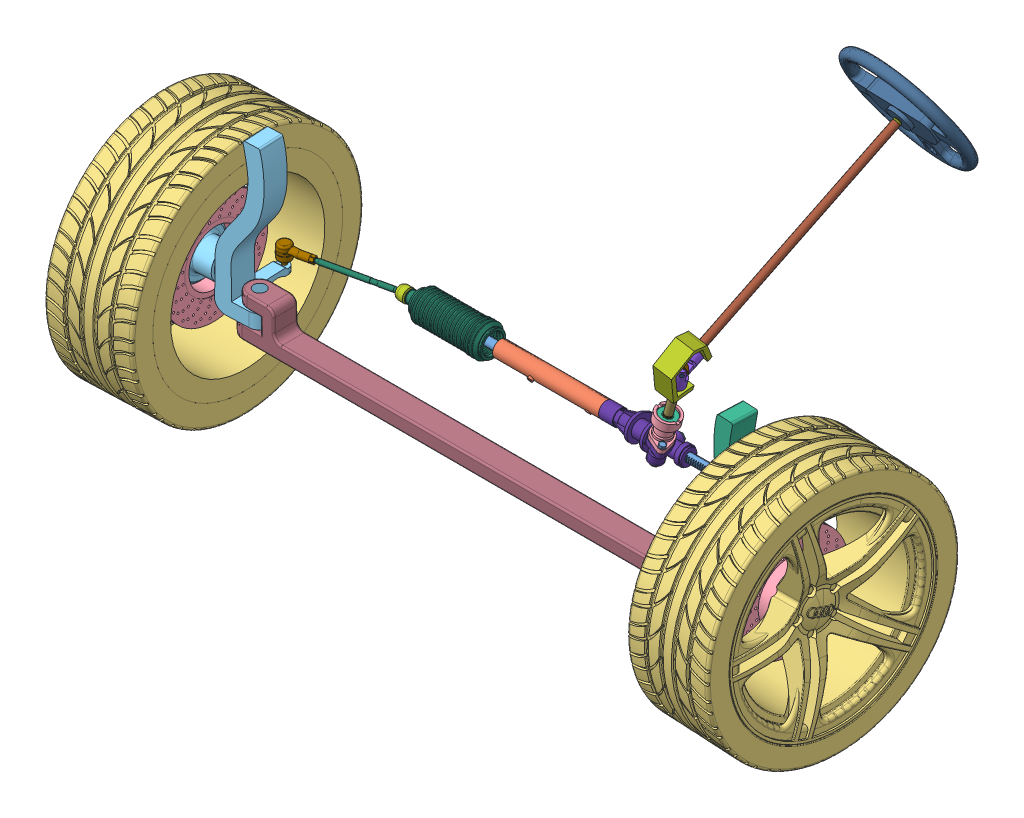
SolidWorks assembly HỆ THỐNG LÁI, configuration Default. Lengths in mm.
Overall size (1991.38 1196.91 1377.29).
45 component instances, 34 part files, 99 mates.
Components (placement in the parent):
- formed hex screw_am-1: formed hex screw_am [B18.2.3.2M - Formed hex screw, M10 x 1.5 x 25 --25WS] at (203.2147 96.225 194.8951) x (-0.267944 -0.963434 0) z (0.029399 -0.008176 0.999534) size (31.63 18.48 16)
- formed hex screw_am-2: formed hex screw_am [B18.2.3.2M - Formed hex screw, M10 x 1.5 x 25 --25WS] at (249.0045 83.4902 243.5967) x (-0.267944 -0.963434 0) z (0.097823 -0.027206 0.994832) size (31.63 18.48 16)
- THƯỚC LÁI-3: THƯỚC LÁI [Default] at (-246.9846 43.7433 199.2709) x (1 0 0) z (0 -0.882001 -0.471248) size (295 48.35 43.5)
- BÁNH XE-1: BÁNH XE [Varsayılan] at (-55.7357 64.8163 360.7964) x (0.047772 -0.300245 -0.952665) z (-0.016934 -0.95386 0.299772) size (668.92 273.92 668.92)
- ĐĨA THẮNG-2: ĐĨA THẮNG [Default] at (-852.1937 65.1305 399.9751) x (0.004037 0.995257 0.097198) z (0.035256 -0.09728 0.994632) size (303 56.33 303)
- BÁNH XE-2: BÁNH XE [Varsayılan] at (-42.761 64.6537 371.2368) x (-0.023989 -0.748 -0.663265) z (-0.02615 0.663699 -0.747543) size (668.92 273.92 668.92)
- KHUNG TREO R-1: KHUNG TREO R [Default] at (-765.1865 65.0792 396.886) x (-0.99937 0.000589 0.035482) z (0.03547 -0.014236 0.999269) size (231.48 449.46 221.1)
- KHUNG TREO L-1: KHUNG TREO L [Default] at (670.2109 63.4994 397.6144) x (0.998715 -0.001812 0.050652) z (0.050673 0.014132 -0.998615) size (231.48 449.46 221.1)
- ĐĨA THẮNG-3: ĐĨA THẮNG [Default] at (753.1662 63.349 401.8216) x (-0.048602 -0.317762 0.946924) z (-0.01438 0.948169 0.317441) size (303 56.33 303)
- CACDANG 5-1: CACDANG 5 [Default] at (259.0901 291.6158 242.3294) x (-0.055622 -0.503507 0.862199) z (0.959177 -0.26676 -0.093904) size (119.51 136.21 49)
- CACDANG 1-2: CACDANG 1 [Default] at (278.0374 289.9791 179.6097) x (-0.173357 0.85529 0.488289) z (-0.055622 -0.503507 0.862199) size (40 40 56)
- CACDANG 2-2: CACDANG 2 [Default] at (284.0824 264.425 226.5167) x (0.640489 0.474538 -0.603811) z (-0.748145 0.208069 -0.630068) size (23 23 23)
- CACDANG 3-1: CACDANG 3 [Default] at (260.5158 270.9792 206.6695) x (0.65777 0.107664 -0.745484) z (0.748145 -0.208069 0.630068) size (10 10 40.8)
- CACDANG 4-1: CACDANG 4 [Default] at (278.9459 249.712 209.5051) x (0.851053 0.379608 -0.362775) z (-0.173357 0.85529 0.488289) size (10 10 14.2)
- CACDANG 4-2: CACDANG 4 [Default] at (274.4733 271.7785 222.103) x (0.851053 0.379608 -0.362775) z (-0.173357 0.85529 0.488289) size (10 10 14.2)
- TRỤC NỐI TRỤC VÍT-2: TRỤC NỐI TRỤC VÍT [Default] at (240.646 141.5713 219.2709) x (0.960852 -0.267226 0.073168) z (0.267944 0.963434 0) size (20 20 100)
- CACDANG 1-3: CACDANG 1 [Default] at (263.1533 222.4998 219.2709) x (0.748145 -0.208069 0.630068) z (0.267944 0.963434 0) size (40 40 56)
- KHUNG GẦM-3: KHUNG GẦM [Default] at (-47.6162 -67.6316 359.9452) x (0.999999 -0.001094 0.000037) z (-0.001093 -0.999898 -0.014206) size (1446 67 117)
- CHỐT HÃM-6: CHỐT HÃM [Default] at (625.5096 48.1445 395.1288) x (0.999999 -0.001094 0.000016) z (-0.001093 -0.999898 -0.014206) size (33.5 33.5 117)
- CHỐT HÃM-5: CHỐT HÃM [Default] at (-720.4896 49.6169 395.0791) x (0.999999 -0.001094 0.000016) z (-0.001093 -0.999898 -0.014206) size (33.5 33.5 117)
- ROTUYN TRONG-1: ROTUYN TRONG [Default] at (-504.6777 43.5088 197.2103) x (-0.9763 -0.000113 0.216421) z (0.160624 -0.670575 0.724244) size (257.66 24 24)
- ROTUYN TRONG-2: ROTUYN TRONG [Default] at (412.1674 43.7741 196.4187) x (0.97478 -0.002427 0.223157) z (0.130993 0.815786 -0.563324) size (257.66 24 24)
- TRỤC VÔ LĂNG 2-3: TRỤC VÔ LĂNG 2 [Default] at (283.9585 343.601 87.7844) x (0.989756 0.085913 0.114023) z (0.055622 0.503507 -0.862199) size (20 20 532)
- VỎ CƠ CẤU LÁI-2: VỎ CƠ CẤU LÁI [Default] at (41.4337 43.7433 199.2709) size (236.3 72.67 100.51)
- TRỤC VÍT-1: TRỤC VÍT [Default] at (206.441 18.5819 219.2709) x (0.686426 -0.190854 -0.701708) z (0.67605 -0.188019 0.712465) size (25.52 146.66 25.52)
- THANH RĂNG-2: THANH RĂNG [Default] at (402.7364 43.7433 199.2709) x (0 -1 -0.000036) z (-1 0 0) size (38 38 898)
- Ổ BI NHỎ-1: Ổ BI NHỎ [Default] at (206.4223 18.5148 219.2709) x (-0.956047 0.26589 0.123602) z (-0.119083 0.033119 -0.992332) size (26 8 26)
- NẮP Ổ BI-1: NẮP Ổ BI [Default] at (201.9775 2.5329 219.2709) x (0.963402 -0.267884 0.009757) z (-0.0094 0.002614 0.999952) size (30.59 16.59 30.59)
- VỎ TRỤC VÍT-1: VỎ TRỤC VÍT [Default] at (224.4762 83.4302 219.2711) x (-0.013584 0.003742 0.999901) z (-0.963339 0.267918 -0.01409) size (68.03 72.52 68.21)
- Ổ BI HÃM-1: Ổ BI HÃM [Default] at (219.596 65.8829 219.2709) x (0.843571 -0.234609 -0.483059) z (0.465396 -0.129433 0.875588) size (37.58 11 37.58)
- Ổ BI LỚN-1: Ổ BI LỚN [Default] at (239.2278 136.4722 219.273) x (-0.596204 0.16584 -0.785517) z (-0.267944 -0.963435 -0.000034) size (47 47 14)
- KHỚP CẦU 3-1: KHỚP CẦU 3 [Default] at (408.7364 43.7474 198.8734) x (-1 0 0) z (0 -0.010312 0.999947) size (48.52 36 36)
- KHỚP CẦU 3-2: KHỚP CẦU 3 [Default] at (-501.2636 43.5076 199.5909) x (1 0 0) z (0 0.593004 -0.8052) size (48.52 36 36)
- KHỚP CẦU-1: KHỚP CẦU [Default] at (408.8899 43.7474 198.8734) x (0 -0.967498 -0.252877) z (0 0.252877 -0.967498) size (28 21.64 28)
- KHỚP CẦU-2: KHỚP CẦU [Default] at (-501.417 43.5076 199.5909) x (0 0.837169 0.546944) z (0 0.546944 -0.837169) size (28 21.64 28)
- ROTUYN NGOÀI-1: ROTUYN NGOÀI [Default] at (693.8678 36.4157 260.8858) x (-0.97478 0.002427 -0.223157) z (-0.223164 -0.003333 0.974775) size (90.98 73 54.28)
- ROTUYN NGOÀI-2: ROTUYN NGOÀI [Default] at (-786.8333 36.8192 259.7307) x (0.9763 0.000113 -0.216421) z (-0.21642 0.003851 -0.976293) size (90.98 73 54.28)
- VÔ LĂNG-2: VÔ LĂNG [Default] at (313.8278 613.9844 -375.2162) x (0.989756 0.085913 0.114023) z (0.055622 0.503507 -0.862199) size (350 350 50.57)
- TRỤC VÔ LĂNG-4: TRỤC VÔ LĂNG [Default] at (278.3989 293.2519 174.0055) x (-0.997646 -0.006666 -0.068253) z (0.055622 0.503507 -0.862199) size (20 20 622.5)
- DẪN HƯỚNG-1: DẪN HƯỚNG [Default] at (217.2671 43.7433 186.497) x (0 0 1) z (-1 0 0) size (16.14 26.77 26.77)
- LÒ XO-1: LÒ XO [Default] at (217.2478 43.7129 169.497) x (-0.923728 -0.383049 0) z (0 0 -1) size (18.46 18.46 19.47)
- NẮP DẪN HƯỚNG-1: NẮP DẪN HƯỚNG [Default] at (217.2671 43.7433 186.7009) x (0.739281 -0.673397 0) z (0.673397 0.739281 0) size (28.57 26.12 28.57)
- CAO SU CHẤN BỤI-1: CAO SU CHẤN BỤI [Default] at (-266.9846 43.7433 199.2709) x (-1 0 0) z (0 -0.974185 -0.22575) size (230.52 87.2 87.2)
- KHỚP NỐI-2: KHỚP NỐI [Default] at (-266.9846 43.7433 199.2709) x (0 0.992312 -0.123763) z (1 0 0) size (50 50 31) (hidden)
- CAO SU CHẤN BỤI-2: CAO SU CHẤN BỤI [Default] at (272.7278 43.7433 199.2709) size (230.52 87.2 87.2) (hidden)
Mates (geometry in assembly coordinates):
- Tangent14: tangent aligned: plane of ĐĨA THẮNG-2 through (-889.1034 -9.4922 393.9849) normal (0.99937 -0.000589 -0.035482); torus of KHUNG TREO R-1
- Concentric17: concentric aligned: cylinder of ĐĨA THẮNG-2 through (-852.1937 65.1305 399.9751) axis (0.99937 -0.000589 -0.035482) radius 35; cone of KHUNG TREO R-1 through (-886.8193 65.1509 401.2044) axis (0.99937 -0.000589 -0.035482)
- Tangent16: tangent anti-aligned: torus of KHUNG TREO L-1; plane of ĐĨA THẮNG-3 through (793.3942 87.1147 332.6577) normal (-0.998715 0.001812 -0.050652)
- Concentric20: concentric aligned: cone of KHUNG TREO L-1 through (791.7639 63.2789 403.7792) axis (-0.998715 0.001812 -0.050652); cylinder of ĐĨA THẮNG-3 through (753.1662 63.349 401.8216) axis (-0.998715 0.001812 -0.050652) radius 35
- Coincident11: coincident anti-aligned: plane of BÁNH XE-1 through (796.9399 63.2696 404.0417) normal (-0.998715 0.001812 -0.050652); plane of ĐĨA THẮNG-3 through (798.6409 74.3912 370.8993) normal (0.998715 -0.001812 0.050652)
- Concentric24: concentric aligned: cylinder of BÁNH XE-1 through (858.6584 10.886 423.646) axis (0.998715 -0.001812 0.050652) radius 13; cylinder of ĐĨA THẮNG-3 through (752.0989 11.0793 418.2416) axis (0.998715 -0.001812 0.050652) radius 13
- Concentric25: concentric aligned: cylinder of BÁNH XE-1 through (858.7984 115.114 424.6142) axis (0.998715 -0.001812 0.050652) radius 13; cylinder of ĐĨA THẮNG-3 through (752.2388 115.3073 419.2098) axis (0.998715 -0.001812 0.050652) radius 13
- Concentric26: concentric aligned: cylinder of BÁNH XE-1 through (861.8758 95.7724 363.2442) axis (0.998715 -0.001812 0.050652) radius 13; cylinder of ĐĨA THẮNG-3 through (755.3163 95.9657 357.8398) axis (0.998715 -0.001812 0.050652) radius 13
- Concentric27: concentric aligned: cylinder of BÁNH XE-1 through (861.7893 31.356 362.6458) axis (0.998715 -0.001812 0.050652) radius 13; cylinder of ĐĨA THẮNG-3 through (755.2298 31.5493 357.2414) axis (0.998715 -0.001812 0.050652) radius 13
- Concentric28: concentric aligned: cylinder of BÁNH XE-1 through (856.8099 62.6513 461.9445) axis (0.998715 -0.001812 0.050652) radius 13; cylinder of ĐĨA THẮNG-3 through (750.2504 62.8446 456.5401) axis (0.998715 -0.001812 0.050652) radius 13
- Lock1: lock: unknown of BÁNH XE-1; unknown of ĐĨA THẮNG-3
- Coincident13: coincident anti-aligned: plane of ĐĨA THẮNG-2 through (-896.1374 30.3223 398.1283) normal (-0.99937 0.000589 0.035482); plane of BÁNH XE-2 through (-895.9961 65.1563 401.5303) normal (0.99937 -0.000589 -0.035482)
- Concentric32: concentric aligned: cylinder of ĐĨA THẮNG-2 through (-853.4872 101.5 359.0061) axis (-0.99937 0.000589 0.035482) radius 13; cylinder of BÁNH XE-2 through (-960.1167 101.5628 362.7919) axis (-0.99937 0.000589 0.035482) radius 13
- Concentric33: concentric aligned: cylinder of ĐĨA THẮNG-2 through (-853.7473 37.3862 352.7446) axis (-0.99937 0.000589 0.035482) radius 13; cylinder of BÁNH XE-2 through (-960.3768 37.449 356.5304) axis (-0.99937 0.000589 0.035482) radius 13
- Concentric34: concentric aligned: cylinder of ĐĨA THẮNG-2 through (-851.6676 11.614 411.7472) axis (-0.99937 0.000589 0.035482) radius 13; cylinder of BÁNH XE-2 through (-958.2971 11.6768 415.533) axis (-0.99937 0.000589 0.035482) radius 13
- Lock2: lock: unknown of ĐĨA THẮNG-2; unknown of BÁNH XE-2
- Concentric170: concentric aligned: cylinder of CACDANG 1-2 through (272.0116 283.9236 229.0367) axis (0.173357 -0.85529 -0.488289) radius 5; cylinder of CACDANG 2-2 through (273.4851 276.6536 224.8862) axis (0.173357 -0.85529 -0.488289) radius 5
- Concentric172: concentric aligned: cylinder of CACDANG 1-2 through (272.0116 283.9236 229.0367) axis (0.173357 -0.85529 -0.488289) radius 5; cylinder of CACDANG 4-1 through (276.4842 261.8571 216.4388) axis (0.173357 -0.85529 -0.488289) radius 5
- Coincident127: coincident anti-aligned: plane of CACDANG 1-2 through (256.1827 261.7826 197.6882) normal (-0.173357 0.85529 0.488289); plane of CACDANG 2-2 through (261.5031 253.9176 213.3536) normal (0.173357 -0.85529 -0.488289)
- Tangent49: tangent aligned: cylinder of CACDANG 1-2 through (274.9225 261.7827 227.8929) axis (0.055622 0.503507 -0.862199) radius 20; plane of CACDANG 4-1 through (278.9459 249.712 209.5051) normal (0.173357 -0.85529 -0.488289)
- Concentric173: concentric aligned: cylinder of CACDANG 1-2 through (272.0116 283.9236 229.0367) axis (0.173357 -0.85529 -0.488289) radius 5; cylinder of CACDANG 4-2 through (272.0116 283.9236 229.0367) axis (0.173357 -0.85529 -0.488289) radius 5
- Tangent51: tangent aligned: cylinder of CACDANG 1-2 through (274.9225 261.7827 227.8929) axis (0.055622 0.503507 -0.862199) radius 20; plane of CACDANG 4-2 through (272.0116 283.9236 229.0367) normal (-0.173357 0.85529 0.488289)
- Parallel34: parallel aligned: line of CACDANG 5-1 through (278.7728 292.7321 179.3009) axis (0.055622 0.503507 -0.862199); line of CACDANG 1-2 through (277.0213 280.7817 195.3593) axis (0.055622 0.503507 -0.862199)
- Concentric180: concentric aligned: cylinder of CACDANG 5-1 through (263.1533 222.4998 219.2709) axis (-0.267944 -0.963434 0) radius 10; cylinder of CACDANG 1-3 through (267.4404 237.9148 219.2709) axis (-0.267944 -0.963434 0) radius 10.1
- Coincident130: coincident anti-aligned: plane of CACDANG 5-1 through (288.5395 215.4396 237.7281) normal (0.267944 0.963434 0); plane of CACDANG 1-3 through (263.1533 222.4998 219.2709) normal (-0.267944 -0.963434 0)
- Concentric181: concentric aligned: cylinder of TRỤC NỐI TRỤC VÍT-2 through (267.4404 237.9148 219.2709) axis (-0.267944 -0.963434 0) radius 10; cylinder of CACDANG 1-3 through (267.4404 237.9148 219.2709) axis (-0.267944 -0.963434 0) radius 10.1
- Coincident131: coincident anti-aligned: plane of TRỤC NỐI TRỤC VÍT-2 through (267.4404 237.9148 219.2709) normal (0.267944 0.963434 0); plane of CACDANG 1-3 through (267.4404 237.9148 219.2709) normal (-0.267944 -0.963434 0)
- Lock35: lock: unknown of TRỤC NỐI TRỤC VÍT-2; unknown of CACDANG 1-3
- Concentric183: concentric aligned: cylinder of CACDANG 2-2 through (284.0824 264.425 226.5167) axis (-0.748145 0.208069 -0.630068) radius 5; cylinder of CACDANG 1-3 through (290.4416 262.6564 231.8723) axis (-0.748145 0.208069 -0.630068) radius 5
- Coincident132: coincident anti-aligned: plane of CACDANG 2-2 through (284.0824 264.425 226.5167) normal (0.748145 -0.208069 0.630068); plane of CACDANG 1-3 through (293.7214 246.175 209.0445) normal (-0.748145 0.208069 -0.630068)
- Concentric184: concentric aligned: cylinder of CACDANG 2-2 through (284.0824 264.425 226.5167) axis (-0.748145 0.208069 -0.630068) radius 5; cylinder of CACDANG 3-1 through (291.0402 262.4899 232.3763) axis (-0.748145 0.208069 -0.630068) radius 5
- Tangent55: tangent aligned: plane of CACDANG 3-1 through (260.5158 270.9792 206.6695) normal (-0.748145 0.208069 -0.630068); cylinder of CACDANG 1-3 through (278.1582 276.4521 219.2709) axis (-0.267944 -0.963434 0) radius 20
- Concentric211: concentric aligned: cylinder of KHUNG TREO R-1 through (-720.6256 -74.7467 393.3123) axis (0.001093 0.999898 0.014206) radius 16.75; cylinder of CHỐT HÃM-5 through (-720.6175 -67.3712 393.417) axis (0.001093 0.999898 0.014206) radius 16.75
- Concentric212: concentric aligned: cylinder of KHUNG GẦM-3 through (-720.6693 -114.7426 392.744) axis (0.001093 0.999898 0.014206) radius 16.75; cylinder of CHỐT HÃM-5 through (-720.6175 -67.3712 393.417) axis (0.001093 0.999898 0.014206) radius 16.75
- Coincident162: coincident anti-aligned: plane of KHUNG TREO R-1 through (-775.3055 -26.8669 362.4108) normal (-0.001093 -0.999898 -0.014206); plane of KHUNG GẦM-3 through (-47.5759 -28.5874 427.5067) normal (0.001093 0.999898 0.014206)
- Coincident163: coincident aligned: plane of KHUNG GẦM-3 through (-47.4918 48.4048 428.6006) normal (0.001093 0.999898 0.014206); plane of CHỐT HÃM-5 through (-720.4896 49.6169 395.0791) normal (0.001093 0.999898 0.014206)
- Concentric222: concentric aligned: cylinder of KHUNG TREO L-1 through (625.3736 -76.2191 393.3619) axis (0.001093 0.999898 0.014206) radius 16.75; cylinder of KHUNG GẦM-3 through (625.3299 -116.215 392.7937) axis (0.001093 0.999898 0.014206) radius 16.75
- Concentric223: concentric aligned: cylinder of KHUNG GẦM-3 through (625.3299 -116.215 392.7937) axis (0.001093 0.999898 0.014206) radius 16.75; cylinder of CHỐT HÃM-6 through (625.3817 -68.8436 393.4667) axis (0.001093 0.999898 0.014206) radius 16.75
- Coincident176: coincident anti-aligned: plane of KHUNG TREO L-1 through (677.2362 -29.4182 430.2023) normal (-0.001093 -0.999898 -0.014206); plane of KHUNG GẦM-3 through (-47.5759 -28.5874 427.5067) normal (0.001093 0.999898 0.014206)
- Coincident177: coincident aligned: plane of KHUNG GẦM-3 through (-47.4918 48.4048 428.6006) normal (0.001093 0.999898 0.014206); plane of CHỐT HÃM-6 through (625.5096 48.1445 395.1288) normal (0.001093 0.999898 0.014206)
- Concentric233: concentric aligned: cylinder of VỎ CƠ CẤU LÁI-2 through (235.5536 123.261 219.2709) axis (-0.267944 -0.963434 0) radius 12.76; cylinder of TRỤC VÍT-1 through (206.441 18.5819 219.2709) axis (-0.267944 -0.963434 0) radius 12.76
- Coincident193: coincident aligned: circle of VỎ CƠ CẤU LÁI-2; cylinder of THANH RĂNG-2 through (-195.2636 43.7433 199.2709) axis (1 0 0) radius 11.5
- Coincident194: coincident anti-aligned: plane of VỎ CƠ CẤU LÁI-2 through (208.5659 26.2223 219.2709) normal (-0.267944 -0.963434 0); plane of Ổ BI NHỎ-1 through (208.5659 26.2223 219.2709) normal (0.267944 0.963434 0)
- Concentric236: concentric anti-aligned: cylinder of VỎ CƠ CẤU LÁI-2 through (207.119 21.0198 219.2709) axis (0.267944 0.963434 0) radius 12.8092; cylinder of Ổ BI NHỎ-1 through (208.5659 26.2223 219.2709) axis (-0.267944 -0.963434 0) radius 13
- Concentric237: concentric anti-aligned: cone of TRỤC VÍT-1 through (208.5846 26.2896 219.2709) axis (0.267944 0.963434 0); cylinder of Ổ BI NHỎ-1 through (208.5659 26.2223 219.2709) axis (-0.267944 -0.963434 0) radius 5
- Lock47: lock: unknown of TRỤC VÍT-1; unknown of Ổ BI NHỎ-1
- Concentric238: concentric aligned: cylinder of VỎ CƠ CẤU LÁI-2 through (204.9466 13.2086 219.2709) axis (0.267944 0.963434 0) radius 15.0252; cone of NẮP Ổ BI-1 through (204.141 10.312 219.2709) axis (0.267944 0.963434 0)
- Tangent56: tangent aligned: plane of VỎ CƠ CẤU LÁI-2 through (206.4223 18.5148 219.2709) normal (-0.267944 -0.963434 0); cone of NẮP Ổ BI-1 through (206.4225 18.5156 219.2709) axis (-0.267944 -0.963434 0)
- Concentric240: concentric anti-aligned: cylinder of VỎ CƠ CẤU LÁI-2 through (230.0793 103.5772 219.2709) axis (-0.267944 -0.963434 0) radius 18.79; cone of Ổ BI HÃM-1 through (222.5436 76.4812 219.2709) axis (0.267944 0.963434 0)
- Concentric241: concentric anti-aligned: cylinder of VỎ TRỤC VÍT-1 through (222.5443 76.4839 219.2709) axis (-0.267944 -0.963434 0) radius 18.79; cone of Ổ BI HÃM-1 through (222.5436 76.4812 219.2709) axis (0.267944 0.963434 0)
- Coincident199: coincident anti-aligned: plane of VỎ CƠ CẤU LÁI-2 through (248.448 64.0899 219.2709) normal (0.267944 0.963434 0); plane of VỎ TRỤC VÍT-1 through (221.2046 71.6667 219.2711) normal (-0.267944 -0.963434 0)
- Parallel35: parallel: plane of VỎ CƠ CẤU LÁI-2 through (159.3918 -25.9872 198.4803) normal (-0.935571 0.260195 0.238759); line of VỎ TRỤC VÍT-1 through (195.5712 78.7957 225.8127) axis (-0.230029 0.063974 -0.971079)
- Coincident204: coincident anti-aligned: plane of VỎ TRỤC VÍT-1 through (235.4766 122.9841 219.2725) normal (0.267944 0.963435 0.000034); plane of Ổ BI LỚN-1 through (235.4766 122.9841 219.2725) normal (-0.267944 -0.963435 -0.000034)
- Concentric244: concentric aligned: cylinder of VỎ TRỤC VÍT-1 through (235.4766 122.9841 219.2725) axis (0.267944 0.963435 0.000034) radius 23.4976; cylinder of Ổ BI LỚN-1 through (235.4766 122.9841 219.2725) axis (0.267944 0.963435 0.000034) radius 23.5
- Concentric246: concentric anti-aligned: cylinder of TRỤC NỐI TRỤC VÍT-2 through (245.7369 159.8766 219.2709) axis (-0.267944 -0.963434 0) radius 7.8; cone of TRỤC VÍT-1 through (240.5297 141.1532 219.2709) axis (0.267944 0.963434 0)
- Tangent57: tangent aligned: plane of TRỤC NỐI TRỤC VÍT-2 through (245.7369 159.8766 219.2709) normal (-0.267944 -0.963434 0); cone of TRỤC VÍT-1 through (245.737 159.8769 219.2709) axis (-0.267944 -0.963434 0)
- Concentric247: concentric aligned: cylinder of formed hex screw_am-1 through (203.2147 96.225 194.8951) axis (0.267944 0.963434 0) radius 5; cylinder of VỎ TRỤC VÍT-1 through (198.1666 78.0738 194.8951) axis (0.267944 0.963434 0) radius 4.95
- Coincident205: coincident anti-aligned: plane of formed hex screw_am-1 through (200.9679 89.9682 178.9026) normal (-0.267944 -0.963434 0); plane of VỎ TRỤC VÍT-1 through (224.4762 83.4302 219.2711) normal (0.267944 0.963434 0)
- Concentric248: concentric aligned: cylinder of formed hex screw_am-2 through (249.0045 83.4902 243.5967) axis (0.267944 0.963434 0) radius 5; cylinder of VỎ TRỤC VÍT-1 through (243.9564 65.3391 243.5967) axis (0.267944 0.963434 0) radius 5.0797
- Coincident206: coincident anti-aligned: plane of formed hex screw_am-2 through (245.6628 77.5379 227.6794) normal (-0.267944 -0.963434 0); plane of VỎ TRỤC VÍT-1 through (224.4762 83.4302 219.2711) normal (0.267944 0.963434 0)
- Coincident215: coincident anti-aligned: plane of THƯỚC LÁI-3 through (48.0154 43.7433 199.2709) normal (1 0 0); plane of VỎ CƠ CẤU LÁI-2 through (48.0154 62.7433 199.2709) normal (-1 0 0)
- Concentric252: concentric aligned: cylinder of THƯỚC LÁI-3 through (48.0154 43.7433 199.2709) axis (-1 0 0) radius 19; cylinder of VỎ CƠ CẤU LÁI-2 through (41.4337 43.7433 199.2709) axis (-1 0 0) radius 17.4989
- Coincident216: coincident aligned: cone of KHỚP CẦU 3-1 through (423.7364 43.7474 198.8734) axis (-1 0 0); cone of KHỚP CẦU-1 through (423.7364 43.7474 198.8734) axis (-1 0 0)
- Coincident217: coincident aligned: cone of KHỚP CẦU 3-2 through (-516.2636 43.5076 199.5909) axis (1 0 0); cone of KHỚP CẦU-2 through (-516.2636 43.5076 199.5909) axis (1 0 0)
- Concentric253: concentric: sphere of ROTUYN TRONG-1; sphere of KHỚP CẦU-2
- Concentric254: concentric aligned: cylinder of THANH RĂNG-2 through (-470.2636 43.7433 199.2709) axis (-1 0 0) radius 8; cylinder of KHỚP CẦU 3-2 through (-492.2636 43.7433 199.2709) axis (-1 0 0) radius 7
- Coincident218: coincident anti-aligned: plane of THANH RĂNG-2 through (-495.2636 43.7433 199.2709) normal (-1 0 0); plane of KHỚP CẦU 3-2 through (-495.2636 43.5076 199.5909) normal (1 0 0)
- Concentric255: concentric: sphere of ROTUYN TRONG-2; sphere of KHỚP CẦU-1
- Concentric256: concentric aligned: cylinder of THANH RĂNG-2 through (377.7364 43.7433 199.2709) axis (1 0 0) radius 8; cylinder of KHỚP CẦU 3-1 through (399.7364 43.7433 199.2709) axis (1 0 0) radius 7
- Concentric257: concentric aligned: cylinder of KHUNG TREO L-1 through (693.7681 -25.0752 260.6527) axis (0.001622 0.999992 0.00379) radius 6; cylinder of ROTUYN NGOÀI-1 through (693.8506 25.7706 260.8454) axis (0.001622 0.999992 0.00379) radius 6.4528
- Concentric258: concentric aligned: cylinder of ROTUYN TRONG-2 through (422.8899 43.7474 198.8734) axis (-0.97478 0.002427 -0.223157) radius 5.88; cylinder of ROTUYN NGOÀI-1 through (659.7614 43.1577 253.1005) axis (-0.97478 0.002427 -0.223157) radius 5.15
- Concentric259: concentric aligned: cylinder of KHUNG TREO R-1 through (-786.8769 -23.4408 259.5027) axis (0.000723 0.999993 0.003784) radius 6; cylinder of ROTUYN NGOÀI-2 through (-786.841 26.1741 259.6905) axis (0.000723 0.999993 0.003784) radius 6.4528
- Concentric260: concentric aligned: cylinder of ROTUYN TRONG-1 through (-515.417 43.5076 199.5909) axis (0.9763 0.000113 -0.216421) radius 5.88; cylinder of ROTUYN NGOÀI-2 through (-752.658 43.4802 252.1812) axis (0.9763 0.000113 -0.216421) radius 5.15
- Coincident220: coincident aligned: plane of ROTUYN TRONG-1 through (-716.5349 43.4843 244.1736) normal (0.9763 0.000113 -0.216421); plane of ROTUYN NGOÀI-2 through (-718.6094 52.0213 234.8197) normal (0.9763 0.000113 -0.216421)
- Coincident221: coincident anti-aligned: plane of THANH RĂNG-2 through (402.7364 43.7433 199.2709) normal (1 0 0); plane of KHỚP CẦU 3-1 through (402.7364 43.7474 198.8734) normal (-1 0 0)
- Coincident222: coincident aligned: plane of ROTUYN TRONG-2 through (623.6945 43.2475 244.8437) normal (-0.97478 0.002427 -0.223157); plane of ROTUYN NGOÀI-1 through (621.5628 51.7154 254.2474) normal (-0.97478 0.002427 -0.223157)
- Parallel36: parallel: plane of THANH RĂNG-2 through (220.9599 60.8848 206.2715) normal (0 -0.000036 1)
- RackPinionMate3: rack pinion = 13.4592 mm: line of THANH RĂNG-2 through (100.5841 34.6189 206.2706) axis (-1 0 0); circle of TRỤC VÍT-1
- Lock49: lock: unknown of TRỤC NỐI TRỤC VÍT-2; unknown of TRỤC VÍT-1
- Coincident232: coincident anti-aligned: plane of TRỤC VÔ LĂNG 2-3 through (313.5497 611.4669 -370.9053) normal (0.055622 0.503507 -0.862199); plane of VÔ LĂNG-2 through (306.1775 609.6554 -372.4387) normal (-0.055622 -0.503507 0.862199)
- Coincident233: coincident anti-aligned: plane of TRỤC VÔ LĂNG 2-3 through (313.6738 605.0429 -374.6487) normal (0.131485 -0.859709 -0.493571); plane of VÔ LĂNG-2 through (315.3681 605.19 -374.4535) normal (-0.131485 0.859709 0.493571)
- Coincident234: coincident anti-aligned: plane of TRỤC VÔ LĂNG 2-3 through (315.814 604.9324 -374.5752) normal (-0.53548 -0.713799 -0.45139); plane of VÔ LĂNG-2 through (315.814 604.9324 -374.5752) normal (0.53548 0.713799 0.45139)
- Coincident238: coincident anti-aligned: plane of TRỤC VÔ LĂNG 2-3 through (311.7698 595.3546 -343.3149) normal (-0.055622 -0.503507 0.862199); plane of TRỤC VÔ LĂNG-4 through (311.7724 595.3563 -343.3137) normal (0.055622 0.503507 -0.862199)
- Coincident239: coincident anti-aligned: plane of TRỤC VÔ LĂNG 2-3 through (304.1525 594.6934 -344.1924) normal (-0.922897 0.355452 0.148039); plane of TRỤC VÔ LĂNG-4 through (304.1533 594.695 -344.1915) normal (0.922897 -0.355452 -0.148039)
- Coincident240: coincident anti-aligned: plane of TRỤC VÔ LĂNG 2-3 through (316.4548 589.9553 -346.1658) normal (0.131485 -0.859709 -0.493571); plane of TRỤC VÔ LĂNG-4 through (316.4586 589.9556 -346.1653) normal (-0.131485 0.859709 0.493571)
- Concentric263: concentric anti-aligned: cylinder of CACDANG 1-2 through (277.1474 281.923 193.4049) axis (0.055622 0.503507 -0.862199) radius 10.1; cylinder of TRỤC VÔ LĂNG-4 through (311.7724 595.3563 -343.3137) axis (-0.055622 -0.503507 0.862199) radius 10
- Coincident241: coincident anti-aligned: plane of CACDANG 1-2 through (277.1474 281.923 193.4049) normal (0.055622 0.503507 -0.862199); plane of TRỤC VÔ LĂNG-4 through (277.1474 281.923 193.4049) normal (-0.055622 -0.503507 0.862199)
- Lock50: lock: unknown of CACDANG 1-2; unknown of TRỤC VÔ LĂNG-4
- Concentric265: concentric aligned: cylinder of THANH RĂNG-2 through (-195.2636 43.7433 199.2709) axis (1 0 0) radius 11.5; cylinder of DẪN HƯỚNG-1 through (233.3448 43.7433 199.2709) axis (1 0 0) radius 11.5
- Concentric266: concentric aligned: cylinder of VỎ CƠ CẤU LÁI-2 through (217.2671 43.7433 253.3215) axis (0 0 -1) radius 14; cylinder of DẪN HƯỚNG-1 through (217.2671 43.7433 186.497) axis (0 0 -1) radius 13.3831
- Coincident242: coincident anti-aligned: plane of DẪN HƯỚNG-1 through (220.9721 43.7433 186.497) normal (0 0 -1); plane of LÒ XO-1 through (211.811 31.4678 186.497) normal (0 0 1)
- Concentric268: concentric anti-aligned: cylinder of VỎ CƠ CẤU LÁI-2 through (217.2671 43.7433 253.3215) axis (0 0 -1) radius 14; cylinder of NẮP DẪN HƯỚNG-1 through (217.2671 43.7433 167.6009) axis (0 0 1) radius 14.285
- Coincident244: coincident anti-aligned: plane of VỎ CƠ CẤU LÁI-2 through (217.2671 43.7433 169.2709) normal (0 0 -1); circle of NẮP DẪN HƯỚNG-1
- Concentric272: concentric aligned: cylinder of THƯỚC LÁI-3 through (48.0154 43.7433 199.2709) axis (-1 0 0) radius 19; cylinder of KHỚP NỐI-2 through (-240.9846 43.7433 199.2709) axis (-1 0 0) radius 19
- Coincident247: coincident anti-aligned: plane of THƯỚC LÁI-3 through (-246.9846 43.7433 199.2709) normal (-1 0 0); plane of KHỚP NỐI-2 through (-246.9846 43.7433 199.2709) normal (1 0 0)
- Concentric273: concentric aligned: cylinder of CAO SU CHẤN BỤI-1 through (-266.9846 43.7433 199.2709) axis (1 0 0) radius 28.5431; cylinder of KHỚP NỐI-2 through (-271.9846 43.7433 199.2709) axis (1 0 0) radius 22
- Coincident248: coincident anti-aligned: plane of CAO SU CHẤN BỤI-1 through (-266.9846 51.4662 165.944) normal (1 0 0); plane of KHỚP NỐI-2 through (-266.9846 43.7433 199.2709) normal (-1 0 0)
- Concentric274: concentric aligned: cylinder of CAO SU CHẤN BỤI-2 through (272.7278 43.7433 199.2709) axis (-1 0 0) radius 28.5431; cylinder of VỎ CƠ CẤU LÁI-2 through (277.72 43.7433 199.2709) axis (-1 0 0) radius 22
- Tangent65: tangent anti-aligned: plane of VỎ CƠ CẤU LÁI-2 through (272.72 62.578 199.2709) normal (1 0 0); torus of CAO SU CHẤN BỤI-2
